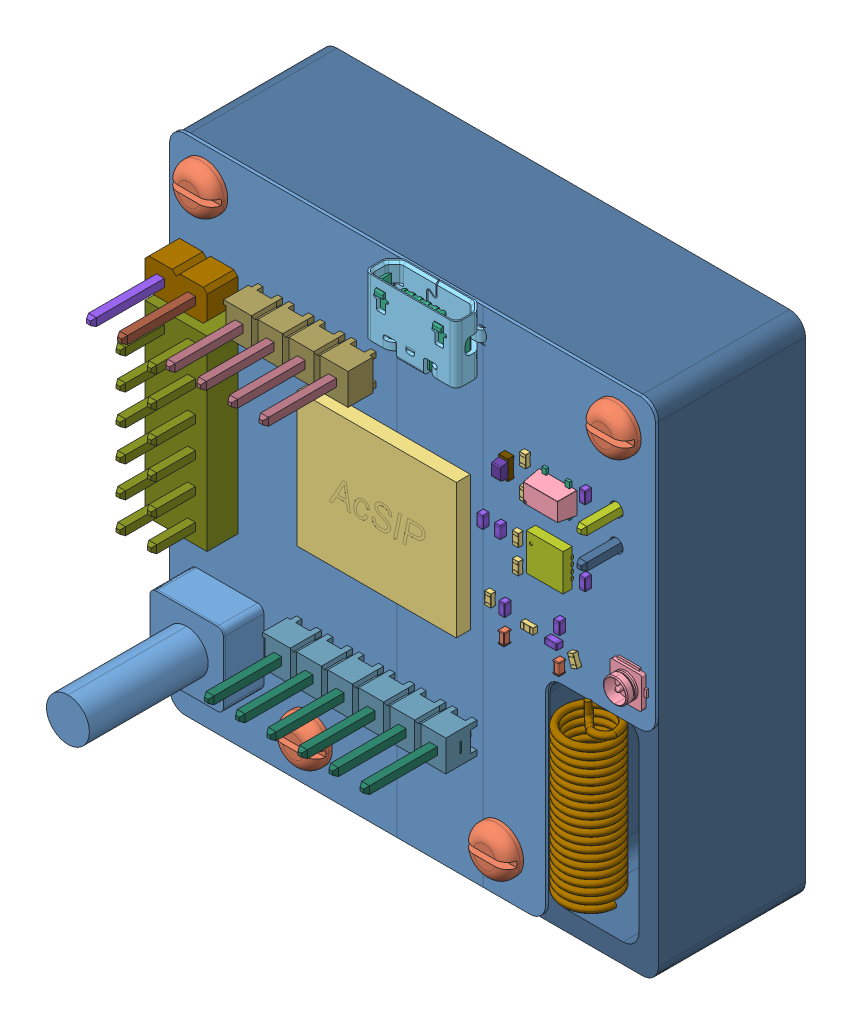
SolidWorks assembly Сборка1, configuration По умолчанию. Lengths in mm.
Overall size (39.69 41.2 25.25).
93 component instances, 28 part files, 3 mates.
Components (placement in the parent):
- PCB1.step-1: PCB1.step [По умолчанию] at (4.9222 -25.9845 21.9043) size (39.69 41.2 21.64)
  - Board.step-1: Board.step [По умолчанию] at origin size (39.69 41.14 0.31)
    - Open CASCADE STEP translator 6.8 2.1.1.step-1: Open CASCADE STEP translator 6.8 2.1.1.step [По умолчанию] at (0 0 -0.2563) size (39.69 41.14 0.31)
  - Open CASCADE STEP translator 6.8 2.2.step-1: Open CASCADE STEP translator 6.8 2.2.step [По умолчанию] at origin size (3.8 3.8 3.31)
    - ______2_______________2__.step-1: ______2_______________2__.step [По умолчанию] at (27 31.4 0) x (-1 0 0) z (0 0 1) size (3.8 3.8 3.31)
  - R3.step-1: R3.step [По умолчанию] at origin size (0.82 1.11 0.41)
    - RESC100X50X40L25N.step-1: RESC100X50X40L25N.step [По умолчанию] at (33.2623 47.9377 0) x (0.34202 -0.939693 0) z (0 0 1) size (1 0.51 0.41)
  - Open CASCADE STEP translator 6.8 2.4.step-1: Open CASCADE STEP translator 6.8 2.4.step [По умолчанию] at origin size (3.8 3.8 3.31)
    - ______2_______________2__.step-1: ______2_______________2__.step [По умолчанию] at (36.6 66 0) x (-1 0 0) z (0 0 1) size (3.8 3.8 3.31)
  - Open CASCADE STEP translator 6.8 2.5.step-1: Open CASCADE STEP translator 6.8 2.5.step [По умолчанию] at origin size (3.8 3.8 3.31)
    - ______2_______________2__.step-1: ______2_______________2__.step [По умолчанию] at (2.85 66.15 0) x (-1 0 0) z (0 0 1) size (3.8 3.8 3.31)
  - Open CASCADE STEP translator 6.8 2.6.step-1: Open CASCADE STEP translator 6.8 2.6.step [По умолчанию] at origin size (3.8 3.8 3.31)
    - ______2_______________2__.step-1: ______2_______________2__.step [По умолчанию] at (11.375 31.4 0) x (-1 0 0) z (0 0 1) size (3.8 3.8 3.31)
  - XW1.step-1: XW1.step [По умолчанию] at origin size (3 3 1.26)
    - U.FL-R-SMT(01).step-1: U.FL-R-SMT(01).step [По умолчанию] at (37.6 48.385 0) x (0 1 0) z (0 0 1) size (3 3 1.26)
  - XS1.step-1: XS1.step [По умолчанию] at origin size (7.5 5.01 3.25)
    - microUSB_1.step-1: microUSB_1.step [По умолчанию] at (25.527 63.125 -5.16) x (-1 0 0) z (0 1 0) size (7.5 3.25 5.01)
      - microUSB_case.step-1: microUSB_case.step [По умолчанию] at (3.4524 5.1465 5.9667) size (7.5 3.05 5)
      - microUSB_inside.step-1: microUSB_inside.step [По умолчанию] at (3.4524 5.4465 5.1667) size (6.9 2.65 4.34)
  - XP5.step-1: XP5.step [По умолчанию] at origin size (2.54 5.08 11.68)
    - 1x2_TH_Vert_100mil.step-1: 1x2_TH_Vert_100mil.step [По умолчанию] at (36.475 57.51 -0.2563) x (0 1 0) z (0 0 -1) size (0.64 0.64 3.3)
    - 1x2_TH_Vert_100mil-0.step-1: 1x2_TH_Vert_100mil-0.step [По умолчанию] at (36.475 57.51 -0.2563) x (0 1 0) z (0 0 -1) size (0.64 0.64 8.38)
    - 1x2_TH_Vert_100mil-1.step-1: 1x2_TH_Vert_100mil-1.step [По умолчанию] at (36.475 57.51 -0.2563) x (0 1 0) z (0 0 -1) size (5.08 2.54 2.5)
    - 1x2_TH_Vert_100mil-2.step-1: 1x2_TH_Vert_100mil-2.step [По умолчанию] at (36.475 57.51 -0.2563) x (0 1 0) z (0 0 -1) size (0.64 0.64 3.3)
    - 1x2_TH_Vert_100mil-3.step-1: 1x2_TH_Vert_100mil-3.step [По умолчанию] at (36.475 57.51 -0.2563) x (0 1 0) z (0 0 -1) size (0.64 0.64 8.38)
  - XP4.step-1: XP4.step [По умолчанию] at origin size (10.29 2.54 10.92)
    - TSW-104-07-G-S.step-1: TSW-104-07-G-S.step [По умолчанию] at (12.0269 60.1249 0) x (1 0 0) z (0 -1 0) size (10.29 10.92 2.54)
      - _TSW-104-07-G-S_body.step-1: _TSW-104-07-G-S_body.step [По умолчанию] at origin size (10.29 2.54 2.54)
      - _T-1S6-07-TSW-1-07-4-S.step-1: _T-1S6-07-TSW-1-07-4-S.step [По умолчанию] at (0 -2.54 0) size (8.51 10.92 0.89)
  - XP3.step-1: XP3.step [По умолчанию] at origin size (15.11 2.54 10.92)
    - TSW-106-07-G-S.step-1: TSW-106-07-G-S.step [По умолчанию] at (19.0001 38.2001 0) x (1 0 0) z (0 -1 0) size (15.11 10.92 2.54)
      - _TSW-107-07-G-S_body.stp.step-1: _TSW-107-07-G-S_body.stp.step [По умолчанию] at origin size (15.11 2.54 2.54)
      - _T-1S6-07-TSW-1-07-7-S.stp.step-1: _T-1S6-07-TSW-1-07-7-S.stp.step [По умолчанию] at (0 -2.54 0) size (14.16 10.92 0.89)
  - XP2.step-1: XP2.step [По умолчанию] at origin size (5.08 2.54 11.68)
    - 1x2_TH_Vert_100mil.step-1: 1x2_TH_Vert_100mil.step [По умолчанию] at (4.3 60.125 0) x (-1 0 0) z (0 0 1) size (0.64 0.64 3.3)
    - 1x2_TH_Vert_100mil-0.step-1: 1x2_TH_Vert_100mil-0.step [По умолчанию] at (4.3 60.125 0) x (-1 0 0) z (0 0 1) size (0.64 0.64 8.38)
    - 1x2_TH_Vert_100mil-1.step-1: 1x2_TH_Vert_100mil-1.step [По умолчанию] at (4.3 60.125 0) x (-1 0 0) z (0 0 1) size (5.08 2.54 2.5)
    - 1x2_TH_Vert_100mil-2.step-1: 1x2_TH_Vert_100mil-2.step [По умолчанию] at (4.3 60.125 0) x (-1 0 0) z (0 0 1) size (0.64 0.64 3.3)
    - 1x2_TH_Vert_100mil-3.step-1: 1x2_TH_Vert_100mil-3.step [По умолчанию] at (4.3 60.125 0) x (-1 0 0) z (0 0 1) size (0.64 0.64 8.38)
  - XP1.step-1: XP1.step [По умолчанию] at origin size (5.08 15.24 8.01)
    - HDRV12W64P254_6X2_1524X508H600.step-1: HDRV12W64P254_6X2_1524X508H600.step [По умолчанию] at (1.79 56.875 0) x (0 -1 0) z (0 0 1) size (15.24 5.08 8.01)
  - VD1.step-1: VD1.step [По умолчанию] at origin size (0.79 1.6 1.1)
    - KP-1608ZGC.step-1: KP-1608ZGC.step [По умолчанию] at (27.7487 58.8839 0) x (0 1 0) z (1 0 0) size (1.2 0.62 0.73)
    - KP-1608ZGC-4.step-1: KP-1608ZGC-4.step [По умолчанию] at (27.7487 58.8839 0) x (0 1 0) z (1 0 0) size (1.6 0.62 0.79)
  - SB1.step-1: SB1.step [По умолчанию] at origin size (6 6 13)
    - KLS7-TS6601.step-1: KLS7-TS6601.step [По умолчанию] at (4.7 35.8 0) x (0 1 0) z (0 0 1) size (6 6 13)
  - R7.step-1: R7.step [По умолчанию] at origin size (0.51 1 0.41)
    - RESC100X50X40L25N.step-1: RESC100X50X40L25N.step [По умолчанию] at (29.2238 57.7088 0) x (0 1 0) z (0 0 1) size (1 0.51 0.41)
  - R5.step-1: R5.step [По умолчанию] at origin size (0.51 1 0.41)
    - RESC100X50X40L25N.step-1: RESC100X50X40L25N.step [По умолчанию] at (28.6248 52.2402 0) x (0 -1 0) z (0 0 1) size (1 0.51 0.41)
  - R6.step-1: R6.step [По умолчанию] at origin size (0.51 1 0.41)
    - RESC100X50X40L25N.step-1: RESC100X50X40L25N.step [По умолчанию] at (29.2238 60.1088 0) x (0 -1 0) z (0 0 1) size (1 0.51 0.41)
  - R4.step-1: R4.step [По умолчанию] at origin size (0.51 1 0.41)
    - RESC100X50X40L25N.step-1: RESC100X50X40L25N.step [По умолчанию] at (28.6248 54.2402 0) x (0 -1 0) z (0 0 1) size (1 0.51 0.41)
  - R2.step-1: R2.step [По умолчанию] at origin size (0.51 1 0.41)
    - RESC100X50X40L25N.step-1: RESC100X50X40L25N.step [По умолчанию] at (26.375 48.835 0) x (0 1 0) z (0 0 1) size (1 0.51 0.41)
  - R1.step-1: R1.step [По умолчанию] at origin size (1 0.51 0.41)
    - RESC100X50X40L25N.step-1: RESC100X50X40L25N.step [По умолчанию] at (29.56 48.385 0) x (1 0 0) z (0 0 1) size (1 0.51 0.41)
  - L2.step-1: L2.step [По умолчанию] at origin size (0.5 1 0.6)
    - INDC100X50X60L10N.step-1: INDC100X50X60L10N.step [По умолчанию] at (32.125 46.935 0) x (0 -1 0) z (0 0 1) size (1 0.5 0.6)
  - L1.step-1: L1.step [По умолчанию] at origin size (0.5 1 0.6)
    - INDC100X50X60L10N.step-1: INDC100X50X60L10N.step [По умолчанию] at (27.65 46.81 0) x (0 -1 0) z (0 0 1) size (1 0.5 0.6)
  - DD1.step-1: DD1.step [По умолчанию] at origin size (13 11 1.14)
    - S7XS.step-1: S7XS.step [По умолчанию] at (18.05 51.075 0) x (1 0 0) z (0 0 1) size (13 11 1.14)
  - DA2.step-1: DA2.step [По умолчанию] at origin size (3.1 2.7 1.45)
    - 5994449712.step-1: 5994449712.step [По умолчанию] at (31.7238 58.9088 0) x (0 1 0) z (0 0 1) size (2.7 3.1 1.45)
      - Body.step-1: Body.step [По умолчанию] at (-0.9 -1.55 0) size (1.8 3.1 1.45)
        - Open_CASCADE_STEP_translator_6.8_1.2.1.step-1: Open_CASCADE_STEP_translator_6.8_1.2.1.step [По умолчанию] at origin size (1.8 3.1 1.45)
      - Open_CASCADE_STEP_translator_6.8_1.1.step-1: Open_CASCADE_STEP_translator_6.8_1.1.step [По умолчанию] at (-0.9 -1.55 0) size (0.24 0.24 0.01)
      - lead.step-1: lead.step [По умолчанию] at (-1.35 -1.1275 0) size (0.57 0.35 0.2)
      - lead.step-2: lead.step [По умолчанию] at (1.35 1.1275 0) x (-1 0 0) z (0 0 1) size (0.57 0.35 0.2)
      - lead.step-3: lead.step [По умолчанию] at (-1.35 -0.1775 0) size (0.57 0.35 0.2)
      - lead.step-4: lead.step [По умолчанию] at (-1.35 0.7725 0) size (0.57 0.35 0.2)
      - lead.step-5: lead.step [По умолчанию] at (1.35 -0.7725 0) x (-1 0 0) z (0 0 1) size (0.57 0.35 0.2)
  - DA1.step-1: DA1.step [По умолчанию] at origin size (3.1 3 0.8)
    - SON9P50_300X300X80L40X25T244X160N.step-1: SON9P50_300X300X80L40X25T244X160N.step [По умолчанию] at (31.4249 54.1901 0) x (0 -1 0) z (0 0 1) size (3 3.1 0.8)
  - C7.step-1: C7.step [По умолчанию] at origin size (0.5 1 0.55)
    - CAPC100X50X55L20N.step-1: CAPC100X50X55L20N.step [По умолчанию] at (34.2238 60.1088 0) x (0 1 0) z (0 0 1) size (1 0.5 0.55)
  - C6.step-1: C6.step [По умолчанию] at origin size (0.5 1 0.55)
    - CAPC100X50X55L20N.step-1: CAPC100X50X55L20N.step [По умолчанию] at (34.2248 53.9652 0) x (0 -1 0) z (0 0 1) size (1 0.5 0.55)
  - C5.step-1: C5.step [По умолчанию] at origin size (0.5 1 0.55)
    - CAPC100X50X55L20N.step-1: CAPC100X50X55L20N.step [По умолчанию] at (25.875 54.2 0) x (0 -1 0) z (0 0 1) size (1 0.5 0.55)
  - C4.step-1: C4.step [По умолчанию] at origin size (0.5 1 0.55)
    - CAPC100X50X55L20N.step-1: CAPC100X50X55L20N.step [По умолчанию] at (27.3 54.2 0) x (0 1 0) z (0 0 1) size (1 0.5 0.55)
  - C3.step-1: C3.step [По умолчанию] at origin size (1 0.5 0.55)
    - CAPC100X50X55L20N.step-1: CAPC100X50X55L20N.step [По умолчанию] at (31.65 48.385 0) x (-1 0 0) z (0 0 1) size (1 0.5 0.55)
  - C2.step-1: C2.step [По умолчанию] at origin size (0.5 1 0.55)
    - CAPC100X50X55L20N.step-1: CAPC100X50X55L20N.step [По умолчанию] at (32.125 49.81 0) x (0 1 0) z (0 0 1) size (1 0.5 0.55)
  - C1.step-1: C1.step [По умолчанию] at origin size (0.5 1 0.55)
    - CAPC100X50X55L20N.step-1: CAPC100X50X55L20N.step [По умолчанию] at (27.65 48.86 0) x (0 1 0) z (0 0 1) size (1 0.5 0.55)
  - Free-Models.step-1: Free-Models.step [По умолчанию] at origin size (4.55 13.83 5.25)
    - Spiral.step-1: Spiral.step [По умолчанию] at (34.525 44.3236 0.3) x (1 0 0) z (0 0 -1) size (4.55 13.83 5.25)
- Bottom.step-1: Bottom.step [По умолчанию] at (53.3875 39.7896 9.658) size (39.54 41.13 12)
Mates (geometry in assembly coordinates):
- Расстояние1: distance = 0.01 mm: plane of Bottom.step-1 through (6.354 3.2155 21.658) normal (0 0 1); plane of PCB1.step-1/Board.step-1/Open CASCADE STEP translator 6.8 2.1.1.step-1 through (6.1922 1.9155 21.648) normal (0 0 -1)
- Совпадение2: coincident: plane of PCB1.step-1/Board.step-1/Open CASCADE STEP translator 6.8 2.1.1.step-1 through (6.1922 43.0405 21.648) normal (0 1 0); plane of Bottom.step-1 through (62.7304 43.0405 21.658) normal (0 1 0)
- Совпадение3: coincident aligned: plane of PCB1.step-1/Board.step-1/Open CASCADE STEP translator 6.8 2.1.1.step-1 through (44.5972 41.7705 21.648) normal (1 0 0); plane of Bottom.step-1 through (44.5972 41.7405 21.658) normal (1 0 0)
